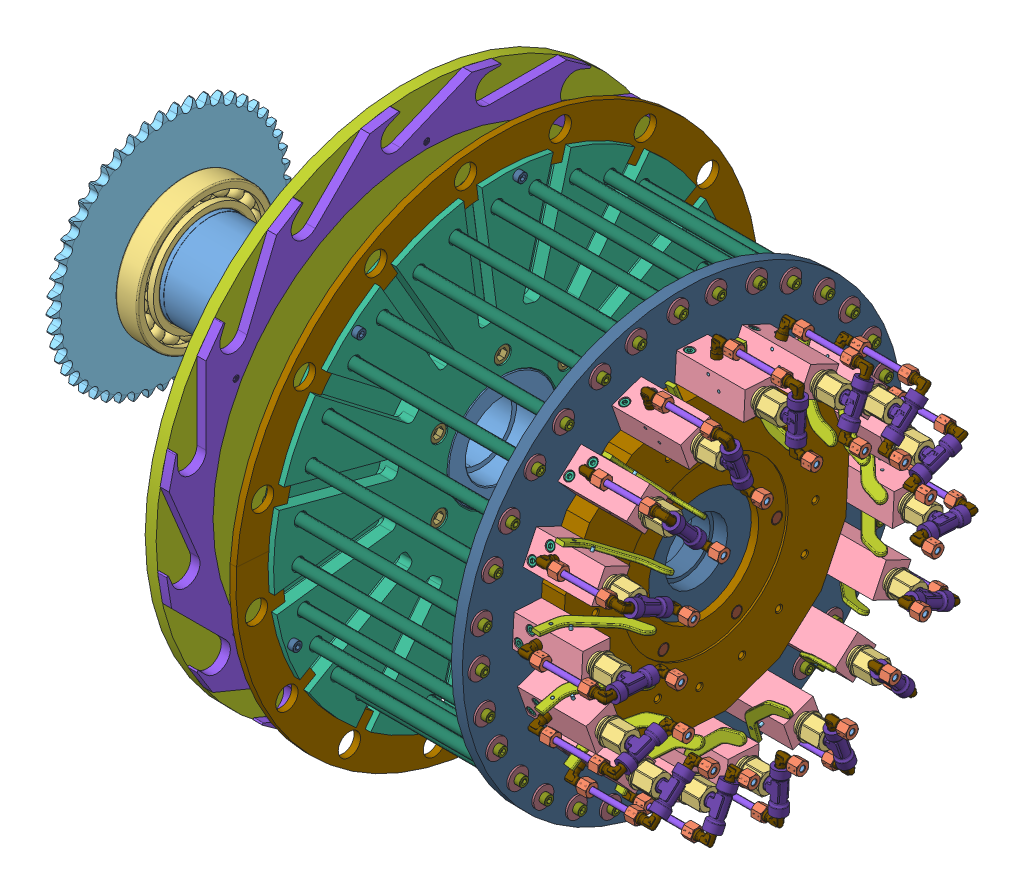
SolidWorks assembly assieme parte rotante, configuration Default. Lengths in mm.
Overall size (749.63 778.63 778.63).
555 component instances, 28 part files, 76 mates.
Components (placement in the parent):
- albero rotazione piatti-1: albero rotazione piatti [Default] at (60.413 18.3637 415) size (415 200 200)
- seger 100mm-1: seger 100mm [KS 1336 E - 100] at (-146.4567 18.3637 415) x (0 0 -1) z (1 0 0) size (107.55 112.98 3)
- SKF - 6020 - 20,DE,NC,20_68-1: SKF - 6020 - 20,DE,NC,20_68 [SKF - 6020 - 20,DE,NC,20_68] at (-131.4567 18.3637 415) x (1 0 0) z (0 -0.434476 -0.900684) size (24 150 150)
- calettatore d95-1: calettatore d95 [Default] at (-173.8867 18.3637 415) size (39.5 135 135)
- Chain wheel ISO - 50Z 10A-1-1: Chain wheel ISO - 50Z 10A-1 [Chain wheel ISO - 50Z 10A-1 --50SB120H25L95.0N] at (-164.8867 18.3637 415) size (28.93 262.06 262.51)
- Disco supporto montaggio e Colonne-1: Disco supporto montaggio e Colonne [Default] at (204.0433 18.3637 415) x (0 -0.866025 -0.5) z (1 0 0) size (499.6 499.6 29)
- SKF - 6020 - 20,DE,NC,20_68-2: SKF - 6020 - 20,DE,NC,20_68 [SKF - 6020 - 20,DE,NC,20_68] at (62.0433 18.3637 415) x (1 0 0) z (0 -0.432628 -0.901573) size (24 150 150)
- piatto rotante porta tappi-1: piatto rotante porta tappi [Default] at (99.0433 18.3637 415) x (0 0 -1) z (1 0 0) size (570 570 20.57)
- disco trasportatore tappi 31-1: disco trasportatore tappi 31 [Default] at (111.0433 18.3637 415) x (0 0.5 -0.866025) z (1 0 0) size (570 570 10.42)
- Distributore Rotante-1: Distributore Rotante [Default] at (425.0433 18.3637 415) x (0 -0.055301 -0.99847) z (1 0 0) size (310 310 25.54)
- disco trascinato porta distributore vuoto-1: disco trascinato porta distributore vuoto [Default] at (400.0433 18.3637 415) x (0 0.055301 0.99847) z (-1 0 0) size (480 480 50)
- m12 35mm-1: m12 35mm [ISO 4762 M12 x 35 - 35N] at (376.0433 -53.0243 378.8925) x (1 0 0) z (0 -0.5 0.866025) size (47 18 18)
- m12 90mm-3: m12 90mm [ISO 4762 M12 x 90 - 90N] at (203.0433 -21.6363 345.718) x (-1 0 0) z (0 -0.5 0.866025) size (102 18 18)
- rondella m6 22mm-1: rondella m6 22mm [Washer ISO 7094 - 6] at (99.0433 -101.6363 207.1539) x (1 0 0) z (0 -1 0) size (2 22 22)
- M6 20mm-1: M6 20mm [ISO 4762 M6 x 20 - 20N] at (91.0433 -101.6363 207.1539) x (1 0 0) z (0 0.5 0.866025) size (26 10 10)
- m12 35mm-2: m12 35mm [ISO 4762 M12 x 35 - 35N] at (376.0433 13.9397 335.1224) x (1 0 0) z (0 -1 0) size (47 18 18)
- m12 35mm-3: m12 35mm [ISO 4762 M12 x 35 - 35N] at (376.0433 85.3277 371.2299) x (1 0 0) z (0 -0.5 -0.866025) size (47 18 18)
- m12 35mm-4: m12 35mm [ISO 4762 M12 x 35 - 35N] at (376.0433 89.7517 451.1075) x (1 0 0) z (0 0.5 -0.866025) size (47 18 18)
- m12 35mm-5: m12 35mm [ISO 4762 M12 x 35 - 35N] at (376.0433 22.7877 494.8776) x (1 0 0) z (0 1 0) size (47 18 18)
- m12 35mm-6: m12 35mm [ISO 4762 M12 x 35 - 35N] at (376.0433 -48.6003 458.7701) x (1 0 0) z (0 0.5 0.866025) size (47 18 18)
- rondella m6 22mm-2: rondella m6 22mm [Washer ISO 7094 - 6] at (99.0433 138.3637 207.1539) x (1 0 0) z (0 -0.5 -0.866025) size (2 22 22)
- rondella m6 22mm-3: rondella m6 22mm [Washer ISO 7094 - 6] at (99.0433 258.3637 415) x (1 0 0) z (0 0.5 -0.866025) size (2 22 22)
- rondella m6 22mm-4: rondella m6 22mm [Washer ISO 7094 - 6] at (99.0433 138.3637 622.8461) x (1 0 0) z (0 1 0) size (2 22 22)
- rondella m6 22mm-5: rondella m6 22mm [Washer ISO 7094 - 6] at (99.0433 -101.6363 622.8461) x (1 0 0) z (0 0.5 0.866025) size (2 22 22)
- rondella m6 22mm-6: rondella m6 22mm [Washer ISO 7094 - 6] at (99.0433 -221.6363 415) x (1 0 0) z (0 -0.5 0.866025) size (2 22 22)
- M6 20mm-2: M6 20mm [ISO 4762 M6 x 20 - 20N] at (91.0433 138.3637 207.1539) x (1 0 0) z (0 -0.5 0.866025) size (26 10 10)
- M6 20mm-3: M6 20mm [ISO 4762 M6 x 20 - 20N] at (91.0433 258.3637 415) x (1 0 0) z (0 -1 0) size (26 10 10)
- M6 20mm-4: M6 20mm [ISO 4762 M6 x 20 - 20N] at (91.0433 138.3637 622.8461) x (1 0 0) z (0 -0.5 -0.866025) size (26 10 10)
- M6 20mm-5: M6 20mm [ISO 4762 M6 x 20 - 20N] at (91.0433 -101.6363 622.8461) x (1 0 0) z (0 0.5 -0.866025) size (26 10 10)
- M6 20mm-6: M6 20mm [ISO 4762 M6 x 20 - 20N] at (91.0433 -221.6363 415) x (1 0 0) z (0 1 0) size (26 10 10)
- m12 90mm-4: m12 90mm [ISO 4762 M12 x 90 - 90N] at (203.0433 58.3637 345.718) x (-1 0 0) z (0 -1 0) size (102 18 18)
- m12 90mm-5: m12 90mm [ISO 4762 M12 x 90 - 90N] at (203.0433 98.3637 415) x (-1 0 0) z (0 -0.5 -0.866025) size (102 18 18)
- m12 90mm-6: m12 90mm [ISO 4762 M12 x 90 - 90N] at (203.0433 58.3637 484.282) x (-1 0 0) z (0 0.5 -0.866025) size (102 18 18)
- m12 90mm-7: m12 90mm [ISO 4762 M12 x 90 - 90N] at (203.0433 -21.6363 484.282) x (-1 0 0) z (0 1 0) size (102 18 18)
- m12 90mm-8: m12 90mm [ISO 4762 M12 x 90 - 90N] at (203.0433 -61.6363 415) x (-1 0 0) z (0 0.5 0.866025) size (102 18 18)
- asta scorrimento carello-1: asta scorrimento carello [Default] at (287.5433 70.1437 197.9013) x (0 0 -1) z (1 0 0) size (12 12 225)
- rondella m6 22mm-7: rondella m6 22mm [Washer ISO 7094 - 6] at (175.0433 70.1437 197.9013) x (1 0 0) z (0 -1 0) size (2 22 22)
- M6 16mm-1: M6 16mm [ISO 4762 M6 x 16 - 16N] at (167.0433 70.1437 197.9013) size (22 10 10)
- M6 16mm-2: M6 16mm [ISO 4762 M6 x 16 - 16N] at (408.0433 70.1437 197.9013) x (-1 0 0) z (0 0 -1) size (22 10 10)
- rondella m6 22mm-8: rondella m6 22mm [Washer ISO 7094 - 6] at (400.0433 70.1437 197.9013) x (-1 0 0) z (0 1 0) size (2 22 22)
- rondella m6 22mm-9: rondella m6 22mm [Washer ISO 7094 - 6] at (175.0433 24.5373 191.8971) x (1 0 0) z (0 -0.965926 -0.258819) size (2 22 22)
- M6 16mm-3: M6 16mm [ISO 4762 M6 x 16 - 16N] at (167.0433 24.5373 191.8971) x (1 0 0) z (0 0.258819 -0.965926) size (22 10 10)
- asta scorrimento carello-2: asta scorrimento carello [Default] at (287.5433 24.5373 191.8971) x (0 0.258819 -0.965926) z (-1 0 0) size (12 12 225)
- rondella m6 22mm-10: rondella m6 22mm [Washer ISO 7094 - 6] at (400.0433 24.5373 191.8971) x (-1 0 0) z (0 0.965926 0.258819) size (2 22 22)
- M6 16mm-4: M6 16mm [ISO 4762 M6 x 16 - 16N] at (408.0433 24.5373 191.8971) x (-1 0 0) z (0 -0.258819 0.965926) size (22 10 10)
- AssiemeValvola-1: AssiemeValvola [Default] at (515.3257 74.6348 254.5832) x (0 -0.331007 0.943628) z (0 0.943628 0.331007) size (90.26 138.63 38)
  - RaccordoT-1: RaccordoT [Default] at origin size (43 29.75 16.5)
  - Raccordo a L-1: Raccordo a L [Default] at (-30 0 0) x (0 -1 0) z (0 0 -1) size (28.34 25.51 14.01)
    - 1809_06_10_01-1: 1809_06_10_01 [Default] at origin size (22.49 23 10)
    - 1809_06_10_02-1: 1809_06_10_02 [Default] at origin size (6.5 8.5 8.5)
    - 1809_06_10_03-1: 1809_06_10_03 [Default] at origin size (11.02 15.01 14.01)
  - Raccordo a L-2: Raccordo a L [Default] at (30 0 0) x (0 1 0) z (0 0 -1) size (28.34 25.51 14.01)
    - 1809_06_10_01-1: 1809_06_10_01 [Default] at origin size (22.49 23 10)
    - 1809_06_10_02-1: 1809_06_10_02 [Default] at origin size (6.5 8.5 8.5)
    - 1809_06_10_03-1: 1809_06_10_03 [Default] at origin size (11.02 15.01 14.01)
  - TappoChiusura-1: TappoChiusura [Default] at (0 -32 0) x (0 -1 0) z (0 0 1) size (38.28 26.74 26.74)
  - CorpoValvola-1: CorpoValvola [Default] at (-15 -115.2824 0) size (30 75 34)
  - Raccordo a L-3: Raccordo a L [Default] at (-30 -88.2824 0) x (0 1 0) z (0 0 1) size (28.34 25.51 14.01)
    - 1809_06_10_01-1: 1809_06_10_01 [Default] at origin size (22.49 23 10)
    - 1809_06_10_02-1: 1809_06_10_02 [Default] at origin size (6.5 8.5 8.5)
    - 1809_06_10_03-1: 1809_06_10_03 [Default] at origin size (11.02 15.01 14.01)
  - Spina_3x38-1: Spina_3x38 [Default] at (0 -68.2824 -21) x (-1 0 0) z (0 0 1) size (3 3 38)
  - Spina_3x38-2: Spina_3x38 [Default] at (-10 -80.2824 -21) x (0.996193 0.087174 0) z (0 0 1) size (3 3 38)
  - M5 40mm-3: M5 40mm [ISO 4762 M5 x 40 - 40N] at (-14.6 -108.7824 9) size (45 8.5 8.5)
  - M5 40mm-2: M5 40mm [ISO 4762 M5 x 40 - 40N] at (-14.6 -96.7824 -9) size (45 8.5 8.5)
  - LevaValvola-1: LevaValvola [Default] at (-24.507 -86.571 -17) x (0.996193 0.087174 0) z (0 0 1) size (77.55 60.2 4)
  - Tubo-1: Tubo [Default] at (-30 -15.9665 0) x (1 0 0) z (0 -1 0) size (6 6 56.4)
- M6 16mm-5: M6 16mm [ISO 4762 M6 x 16 - 16N] at (167.0433 -16.8778 194.6116) x (1 0 0) z (0 0.382683 0.92388) size (22 10 10)
- M6 16mm-6: M6 16mm [ISO 4762 M6 x 16 - 16N] at (167.0433 -98.5342 224.874) x (1 0 0) z (0 0.707107 0.707107) size (22 10 10)
- M6 16mm-7: M6 16mm [ISO 4762 M6 x 16 - 16N] at (167.0433 -162.3939 284.0814) x (1 0 0) z (0 0.92388 0.382683) size (22 10 10)
- M6 16mm-8: M6 16mm [ISO 4762 M6 x 16 - 16N] at (167.0433 -198.735 363.22) x (1 0 0) z (0 1 0) size (22 10 10)
- M6 16mm-9: M6 16mm [ISO 4762 M6 x 16 - 16N] at (167.0433 -202.0247 450.2415) x (1 0 0) z (0 0.92388 -0.382683) size (22 10 10)
- M6 16mm-10: M6 16mm [ISO 4762 M6 x 16 - 16N] at (167.0433 -171.7623 531.8979) x (1 0 0) z (0 0.707107 -0.707107) size (22 10 10)
- M6 16mm-11: M6 16mm [ISO 4762 M6 x 16 - 16N] at (167.0433 -112.5549 595.7576) x (1 0 0) z (0 0.382683 -0.92388) size (22 10 10)
- M6 16mm-12: M6 16mm [ISO 4762 M6 x 16 - 16N] at (167.0433 -33.4163 632.0987) x (1 0 0) z (0 0 -1) size (22 10 10)
- M6 16mm-13: M6 16mm [ISO 4762 M6 x 16 - 16N] at (167.0433 53.6052 635.3884) x (1 0 0) z (0 -0.382683 -0.92388) size (22 10 10)
- M6 16mm-14: M6 16mm [ISO 4762 M6 x 16 - 16N] at (167.0433 135.2616 605.126) x (1 0 0) z (0 -0.707107 -0.707107) size (22 10 10)
- M6 16mm-15: M6 16mm [ISO 4762 M6 x 16 - 16N] at (167.0433 199.1213 545.9186) x (1 0 0) z (0 -0.92388 -0.382683) size (22 10 10)
- M6 16mm-16: M6 16mm [ISO 4762 M6 x 16 - 16N] at (167.0433 235.4624 466.78) x (1 0 0) z (0 -1 0) size (22 10 10)
- M6 16mm-17: M6 16mm [ISO 4762 M6 x 16 - 16N] at (167.0433 238.7521 379.7585) x (1 0 0) z (0 -0.92388 0.382683) size (22 10 10)
- M6 16mm-18: M6 16mm [ISO 4762 M6 x 16 - 16N] at (167.0433 208.4897 298.1021) x (1 0 0) z (0 -0.707107 0.707107) size (22 10 10)
- M6 16mm-19: M6 16mm [ISO 4762 M6 x 16 - 16N] at (167.0433 149.2823 234.2424) x (1 0 0) z (0 -0.382683 0.92388) size (22 10 10)
- rondella m6 22mm-11: rondella m6 22mm [Washer ISO 7094 - 6] at (175.0433 -16.8778 194.6116) x (1 0 0) z (0 -0.92388 0.382683) size (2 22 22)
- rondella m6 22mm-12: rondella m6 22mm [Washer ISO 7094 - 6] at (175.0433 -98.5342 224.874) x (1 0 0) z (0 -0.707107 0.707107) size (2 22 22)
- rondella m6 22mm-13: rondella m6 22mm [Washer ISO 7094 - 6] at (175.0433 -162.3939 284.0814) x (1 0 0) z (0 -0.382683 0.92388) size (2 22 22)
- rondella m6 22mm-14: rondella m6 22mm [Washer ISO 7094 - 6] at (175.0433 -198.735 363.22) size (2 22 22)
- rondella m6 22mm-15: rondella m6 22mm [Washer ISO 7094 - 6] at (175.0433 -202.0247 450.2415) x (1 0 0) z (0 0.382683 0.92388) size (2 22 22)
- rondella m6 22mm-16: rondella m6 22mm [Washer ISO 7094 - 6] at (175.0433 -171.7623 531.8979) x (1 0 0) z (0 0.707107 0.707107) size (2 22 22)
- rondella m6 22mm-17: rondella m6 22mm [Washer ISO 7094 - 6] at (175.0433 -112.5549 595.7576) x (1 0 0) z (0 0.92388 0.382683) size (2 22 22)
- rondella m6 22mm-18: rondella m6 22mm [Washer ISO 7094 - 6] at (175.0433 -33.4163 632.0987) x (1 0 0) z (0 1 0) size (2 22 22)
- rondella m6 22mm-19: rondella m6 22mm [Washer ISO 7094 - 6] at (175.0433 53.6052 635.3884) x (1 0 0) z (0 0.92388 -0.382683) size (2 22 22)
- rondella m6 22mm-20: rondella m6 22mm [Washer ISO 7094 - 6] at (175.0433 135.2616 605.126) x (1 0 0) z (0 0.707107 -0.707107) size (2 22 22)
- rondella m6 22mm-21: rondella m6 22mm [Washer ISO 7094 - 6] at (175.0433 199.1213 545.9186) x (1 0 0) z (0 0.382683 -0.92388) size (2 22 22)
- rondella m6 22mm-22: rondella m6 22mm [Washer ISO 7094 - 6] at (175.0433 235.4624 466.78) x (1 0 0) z (0 0 -1) size (2 22 22)
- rondella m6 22mm-23: rondella m6 22mm [Washer ISO 7094 - 6] at (175.0433 238.7521 379.7585) x (1 0 0) z (0 -0.382683 -0.92388) size (2 22 22)
- rondella m6 22mm-24: rondella m6 22mm [Washer ISO 7094 - 6] at (175.0433 208.4897 298.1021) x (1 0 0) z (0 -0.707107 -0.707107) size (2 22 22)
- rondella m6 22mm-25: rondella m6 22mm [Washer ISO 7094 - 6] at (175.0433 149.2823 234.2424) x (1 0 0) z (0 -0.92388 -0.382683) size (2 22 22)
- asta scorrimento carello-3: asta scorrimento carello [Default] at (287.5433 -16.8778 194.6116) x (0 -0.382683 -0.92388) z (1 0 0) size (12 12 225)
- asta scorrimento carello-4: asta scorrimento carello [Default] at (287.5433 -98.5342 224.874) x (0 -0.707107 -0.707107) z (1 0 0) size (12 12 225)
- asta scorrimento carello-5: asta scorrimento carello [Default] at (287.5433 -162.3939 284.0814) x (0 -0.92388 -0.382683) z (1 0 0) size (12 12 225)
- asta scorrimento carello-6: asta scorrimento carello [Default] at (287.5433 -198.735 363.22) x (0 -1 0) z (1 0 0) size (12 12 225)
- asta scorrimento carello-7: asta scorrimento carello [Default] at (287.5433 -202.0247 450.2415) x (0 -0.92388 0.382683) z (1 0 0) size (12 12 225)
- asta scorrimento carello-8: asta scorrimento carello [Default] at (287.5433 -171.7623 531.8979) x (0 -0.707107 0.707107) z (1 0 0) size (12 12 225)
- asta scorrimento carello-9: asta scorrimento carello [Default] at (287.5433 -112.5549 595.7576) x (0 -0.382683 0.92388) z (1 0 0) size (12 12 225)
- asta scorrimento carello-10: asta scorrimento carello [Default] at (287.5433 -33.4163 632.0987) x (0 0 1) z (1 0 0) size (12 12 225)
- asta scorrimento carello-11: asta scorrimento carello [Default] at (287.5433 53.6052 635.3884) x (0 0.382683 0.92388) z (1 0 0) size (12 12 225)
- asta scorrimento carello-12: asta scorrimento carello [Default] at (287.5433 135.2616 605.126) x (0 0.707107 0.707107) z (1 0 0) size (12 12 225)
- asta scorrimento carello-13: asta scorrimento carello [Default] at (287.5433 199.1213 545.9186) x (0 0.92388 0.382683) z (1 0 0) size (12 12 225)
- asta scorrimento carello-14: asta scorrimento carello [Default] at (287.5433 235.4624 466.78) x (0 1 0) z (1 0 0) size (12 12 225)
- asta scorrimento carello-15: asta scorrimento carello [Default] at (287.5433 238.7521 379.7585) x (0 0.92388 -0.382683) z (1 0 0) size (12 12 225)
- asta scorrimento carello-16: asta scorrimento carello [Default] at (287.5433 208.4897 298.1021) x (0 0.707107 -0.707107) z (1 0 0) size (12 12 225)
- asta scorrimento carello-17: asta scorrimento carello [Default] at (287.5433 149.2823 234.2424) x (0 0.382683 -0.92388) z (1 0 0) size (12 12 225)
- M6 16mm-20: M6 16mm [ISO 4762 M6 x 16 - 16N] at (408.0433 -16.8778 194.6116) x (-1 0 0) z (0 -0.382683 -0.92388) size (22 10 10)
- M6 16mm-21: M6 16mm [ISO 4762 M6 x 16 - 16N] at (408.0433 -98.5342 224.874) x (-1 0 0) z (0 -0.707107 -0.707107) size (22 10 10)
- M6 16mm-22: M6 16mm [ISO 4762 M6 x 16 - 16N] at (408.0433 -162.3939 284.0814) x (-1 0 0) z (0 -0.92388 -0.382683) size (22 10 10)
- M6 16mm-23: M6 16mm [ISO 4762 M6 x 16 - 16N] at (408.0433 -198.735 363.22) x (-1 0 0) z (0 -1 0) size (22 10 10)
- M6 16mm-24: M6 16mm [ISO 4762 M6 x 16 - 16N] at (408.0433 -202.0247 450.2415) x (-1 0 0) z (0 -0.92388 0.382683) size (22 10 10)
- M6 16mm-25: M6 16mm [ISO 4762 M6 x 16 - 16N] at (408.0433 -171.7623 531.8979) x (-1 0 0) z (0 -0.707107 0.707107) size (22 10 10)
- M6 16mm-26: M6 16mm [ISO 4762 M6 x 16 - 16N] at (408.0433 -112.5549 595.7576) x (-1 0 0) z (0 -0.382683 0.92388) size (22 10 10)
- M6 16mm-27: M6 16mm [ISO 4762 M6 x 16 - 16N] at (408.0433 -33.4163 632.0987) x (-1 0 0) z (0 0 1) size (22 10 10)
- M6 16mm-28: M6 16mm [ISO 4762 M6 x 16 - 16N] at (408.0433 53.6052 635.3884) x (-1 0 0) z (0 0.382683 0.92388) size (22 10 10)
- M6 16mm-29: M6 16mm [ISO 4762 M6 x 16 - 16N] at (408.0433 135.2616 605.126) x (-1 0 0) z (0 0.707107 0.707107) size (22 10 10)
- M6 16mm-30: M6 16mm [ISO 4762 M6 x 16 - 16N] at (408.0433 199.1213 545.9186) x (-1 0 0) z (0 0.92388 0.382683) size (22 10 10)
- M6 16mm-31: M6 16mm [ISO 4762 M6 x 16 - 16N] at (408.0433 235.4624 466.78) x (-1 0 0) z (0 1 0) size (22 10 10)
- M6 16mm-32: M6 16mm [ISO 4762 M6 x 16 - 16N] at (408.0433 238.7521 379.7585) x (-1 0 0) z (0 0.92388 -0.382683) size (22 10 10)
- M6 16mm-33: M6 16mm [ISO 4762 M6 x 16 - 16N] at (408.0433 208.4897 298.1021) x (-1 0 0) z (0 0.707107 -0.707107) size (22 10 10)
- M6 16mm-34: M6 16mm [ISO 4762 M6 x 16 - 16N] at (408.0433 149.2823 234.2424) x (-1 0 0) z (0 0.382683 -0.92388) size (22 10 10)
- rondella m6 22mm-26: rondella m6 22mm [Washer ISO 7094 - 6] at (400.0433 -16.8778 194.6116) x (-1 0 0) z (0 0.92388 -0.382683) size (2 22 22)
- rondella m6 22mm-27: rondella m6 22mm [Washer ISO 7094 - 6] at (400.0433 -98.5342 224.874) x (-1 0 0) z (0 0.707107 -0.707107) size (2 22 22)
- rondella m6 22mm-28: rondella m6 22mm [Washer ISO 7094 - 6] at (400.0433 -162.3939 284.0814) x (-1 0 0) z (0 0.382683 -0.92388) size (2 22 22)
- rondella m6 22mm-29: rondella m6 22mm [Washer ISO 7094 - 6] at (400.0433 -198.735 363.22) x (-1 0 0) z (0 0 -1) size (2 22 22)
- rondella m6 22mm-30: rondella m6 22mm [Washer ISO 7094 - 6] at (400.0433 -202.0247 450.2415) x (-1 0 0) z (0 -0.382683 -0.92388) size (2 22 22)
- rondella m6 22mm-31: rondella m6 22mm [Washer ISO 7094 - 6] at (400.0433 -171.7623 531.8979) x (-1 0 0) z (0 -0.707107 -0.707107) size (2 22 22)
- rondella m6 22mm-32: rondella m6 22mm [Washer ISO 7094 - 6] at (400.0433 -112.5549 595.7576) x (-1 0 0) z (0 -0.92388 -0.382683) size (2 22 22)
- rondella m6 22mm-33: rondella m6 22mm [Washer ISO 7094 - 6] at (400.0433 -33.4163 632.0987) x (-1 0 0) z (0 -1 0) size (2 22 22)
- rondella m6 22mm-34: rondella m6 22mm [Washer ISO 7094 - 6] at (400.0433 53.6052 635.3884) x (-1 0 0) z (0 -0.92388 0.382683) size (2 22 22)
- rondella m6 22mm-35: rondella m6 22mm [Washer ISO 7094 - 6] at (400.0433 135.2616 605.126) x (-1 0 0) z (0 -0.707107 0.707107) size (2 22 22)
- rondella m6 22mm-36: rondella m6 22mm [Washer ISO 7094 - 6] at (400.0433 199.1213 545.9186) x (-1 0 0) z (0 -0.382683 0.92388) size (2 22 22)
- rondella m6 22mm-37: rondella m6 22mm [Washer ISO 7094 - 6] at (400.0433 235.4624 466.78) x (-1 0 0) z (0 0 1) size (2 22 22)
- rondella m6 22mm-38: rondella m6 22mm [Washer ISO 7094 - 6] at (400.0433 238.7521 379.7585) x (-1 0 0) z (0 0.382683 0.92388) size (2 22 22)
- rondella m6 22mm-39: rondella m6 22mm [Washer ISO 7094 - 6] at (400.0433 208.4897 298.1021) x (-1 0 0) z (0 0.707107 0.707107) size (2 22 22)
- rondella m6 22mm-40: rondella m6 22mm [Washer ISO 7094 - 6] at (400.0433 149.2823 234.2424) x (-1 0 0) z (0 0.92388 0.382683) size (2 22 22)
- rondella m6 22mm-41: rondella m6 22mm [Washer ISO 7094 - 6] at (175.0433 -61.3104 206.5173) x (1 0 0) z (0 -0.991445 0.130526) size (2 22 22)
- rondella m6 22mm-42: rondella m6 22mm [Washer ISO 7094 - 6] at (175.0433 -135.0285 252.8771) x (1 0 0) z (0 -0.866025 0.5) size (2 22 22)
- rondella m6 22mm-43: rondella m6 22mm [Washer ISO 7094 - 6] at (175.0433 -185.3939 323.9186) x (1 0 0) z (0 -0.608761 0.793353) size (2 22 22)
- rondella m6 22mm-44: rondella m6 22mm [Washer ISO 7094 - 6] at (175.0433 -204.7392 408.8264) x (1 0 0) z (0 -0.258819 0.965926) size (2 22 22)
- rondella m6 22mm-45: rondella m6 22mm [Washer ISO 7094 - 6] at (175.0433 -190.119 494.6741) x (1 0 0) z (0 0.130526 0.991445) size (2 22 22)
- rondella m6 22mm-46: rondella m6 22mm [Washer ISO 7094 - 6] at (175.0433 -143.7592 568.3922) x (1 0 0) z (0 0.5 0.866025) size (2 22 22)
- rondella m6 22mm-47: rondella m6 22mm [Washer ISO 7094 - 6] at (175.0433 -72.7177 618.7576) x (1 0 0) z (0 0.793353 0.608761) size (2 22 22)
- rondella m6 22mm-48: rondella m6 22mm [Washer ISO 7094 - 6] at (175.0433 12.1901 638.1029) x (1 0 0) z (0 0.965926 0.258819) size (2 22 22)
- rondella m6 22mm-49: rondella m6 22mm [Washer ISO 7094 - 6] at (175.0433 98.0378 623.4827) x (1 0 0) z (0 0.991445 -0.130526) size (2 22 22)
- rondella m6 22mm-50: rondella m6 22mm [Washer ISO 7094 - 6] at (175.0433 171.7559 577.1229) x (1 0 0) z (0 0.866025 -0.5) size (2 22 22)
- rondella m6 22mm-51: rondella m6 22mm [Washer ISO 7094 - 6] at (175.0433 222.1213 506.0814) x (1 0 0) z (0 0.608761 -0.793353) size (2 22 22)
- rondella m6 22mm-52: rondella m6 22mm [Washer ISO 7094 - 6] at (175.0433 241.4666 421.1736) x (1 0 0) z (0 0.258819 -0.965926) size (2 22 22)
- rondella m6 22mm-53: rondella m6 22mm [Washer ISO 7094 - 6] at (175.0433 226.8464 335.3259) x (1 0 0) z (0 -0.130526 -0.991445) size (2 22 22)
- rondella m6 22mm-54: rondella m6 22mm [Washer ISO 7094 - 6] at (175.0433 180.4866 261.6078) x (1 0 0) z (0 -0.5 -0.866025) size (2 22 22)
- rondella m6 22mm-55: rondella m6 22mm [Washer ISO 7094 - 6] at (175.0433 109.4451 211.2424) x (1 0 0) z (0 -0.793353 -0.608761) size (2 22 22)
- M6 16mm-35: M6 16mm [ISO 4762 M6 x 16 - 16N] at (167.0433 -61.3104 206.5173) x (1 0 0) z (0 -0.130526 -0.991445) size (22 10 10)
- M6 16mm-36: M6 16mm [ISO 4762 M6 x 16 - 16N] at (167.0433 -135.0285 252.8771) x (1 0 0) z (0 -0.5 -0.866025) size (22 10 10)
- M6 16mm-37: M6 16mm [ISO 4762 M6 x 16 - 16N] at (167.0433 -185.3939 323.9186) x (1 0 0) z (0 -0.793353 -0.608761) size (22 10 10)
- M6 16mm-38: M6 16mm [ISO 4762 M6 x 16 - 16N] at (167.0433 -204.7392 408.8264) x (1 0 0) z (0 -0.965926 -0.258819) size (22 10 10)
- M6 16mm-39: M6 16mm [ISO 4762 M6 x 16 - 16N] at (167.0433 -190.119 494.6741) x (1 0 0) z (0 -0.991445 0.130526) size (22 10 10)
- M6 16mm-40: M6 16mm [ISO 4762 M6 x 16 - 16N] at (167.0433 -143.7592 568.3922) x (1 0 0) z (0 -0.866025 0.5) size (22 10 10)
- M6 16mm-41: M6 16mm [ISO 4762 M6 x 16 - 16N] at (167.0433 -72.7177 618.7576) x (1 0 0) z (0 -0.608761 0.793353) size (22 10 10)
- M6 16mm-42: M6 16mm [ISO 4762 M6 x 16 - 16N] at (167.0433 12.1901 638.1029) x (1 0 0) z (0 -0.258819 0.965926) size (22 10 10)
- M6 16mm-43: M6 16mm [ISO 4762 M6 x 16 - 16N] at (167.0433 98.0378 623.4827) x (1 0 0) z (0 0.130526 0.991445) size (22 10 10)
- M6 16mm-44: M6 16mm [ISO 4762 M6 x 16 - 16N] at (167.0433 171.7559 577.1229) x (1 0 0) z (0 0.5 0.866025) size (22 10 10)
- M6 16mm-45: M6 16mm [ISO 4762 M6 x 16 - 16N] at (167.0433 222.1213 506.0814) x (1 0 0) z (0 0.793353 0.608761) size (22 10 10)
- M6 16mm-46: M6 16mm [ISO 4762 M6 x 16 - 16N] at (167.0433 241.4666 421.1736) x (1 0 0) z (0 0.965926 0.258819) size (22 10 10)
- M6 16mm-47: M6 16mm [ISO 4762 M6 x 16 - 16N] at (167.0433 226.8464 335.3259) x (1 0 0) z (0 0.991445 -0.130526) size (22 10 10)
- M6 16mm-48: M6 16mm [ISO 4762 M6 x 16 - 16N] at (167.0433 180.4866 261.6078) x (1 0 0) z (0 0.866025 -0.5) size (22 10 10)
- M6 16mm-49: M6 16mm [ISO 4762 M6 x 16 - 16N] at (167.0433 109.4451 211.2424) x (1 0 0) z (0 0.608761 -0.793353) size (22 10 10)
- asta scorrimento carello-18: asta scorrimento carello [Default] at (287.5433 -61.3104 206.5173) x (0 -0.130526 -0.991445) z (-1 0 0) size (12 12 225)
- asta scorrimento carello-19: asta scorrimento carello [Default] at (287.5433 -135.0285 252.8771) x (0 -0.5 -0.866025) z (-1 0 0) size (12 12 225)
- asta scorrimento carello-20: asta scorrimento carello [Default] at (287.5433 -185.3939 323.9186) x (0 -0.793353 -0.608761) z (-1 0 0) size (12 12 225)
- asta scorrimento carello-21: asta scorrimento carello [Default] at (287.5433 -204.7392 408.8264) x (0 -0.965926 -0.258819) z (-1 0 0) size (12 12 225)
- asta scorrimento carello-22: asta scorrimento carello [Default] at (287.5433 -190.119 494.6741) x (0 -0.991445 0.130526) z (-1 0 0) size (12 12 225)
- asta scorrimento carello-23: asta scorrimento carello [Default] at (287.5433 -143.7592 568.3922) x (0 -0.866025 0.5) z (-1 0 0) size (12 12 225)
- asta scorrimento carello-24: asta scorrimento carello [Default] at (287.5433 -72.7177 618.7576) x (0 -0.608761 0.793353) z (-1 0 0) size (12 12 225)
- asta scorrimento carello-25: asta scorrimento carello [Default] at (287.5433 12.1901 638.1029) x (0 -0.258819 0.965926) z (-1 0 0) size (12 12 225)
- asta scorrimento carello-26: asta scorrimento carello [Default] at (287.5433 98.0378 623.4827) x (0 0.130526 0.991445) z (-1 0 0) size (12 12 225)
- asta scorrimento carello-27: asta scorrimento carello [Default] at (287.5433 171.7559 577.1229) x (0 0.5 0.866025) z (-1 0 0) size (12 12 225)
- asta scorrimento carello-28: asta scorrimento carello [Default] at (287.5433 222.1213 506.0814) x (0 0.793353 0.608761) z (-1 0 0) size (12 12 225)
- asta scorrimento carello-29: asta scorrimento carello [Default] at (287.5433 241.4666 421.1736) x (0 0.965926 0.258819) z (-1 0 0) size (12 12 225)
- asta scorrimento carello-30: asta scorrimento carello [Default] at (287.5433 226.8464 335.3259) x (0 0.991445 -0.130526) z (-1 0 0) size (12 12 225)
- asta scorrimento carello-31: asta scorrimento carello [Default] at (287.5433 180.4866 261.6078) x (0 0.866025 -0.5) z (-1 0 0) size (12 12 225)
- asta scorrimento carello-32: asta scorrimento carello [Default] at (287.5433 109.4451 211.2424) x (0 0.608761 -0.793353) z (-1 0 0) size (12 12 225)
- rondella m6 22mm-56: rondella m6 22mm [Washer ISO 7094 - 6] at (400.0433 -61.3104 206.5173) x (-1 0 0) z (0 0.991445 -0.130526) size (2 22 22)
- rondella m6 22mm-57: rondella m6 22mm [Washer ISO 7094 - 6] at (400.0433 -135.0285 252.8771) x (-1 0 0) z (0 0.866025 -0.5) size (2 22 22)
- rondella m6 22mm-58: rondella m6 22mm [Washer ISO 7094 - 6] at (400.0433 -185.3939 323.9186) x (-1 0 0) z (0 0.608761 -0.793353) size (2 22 22)
- rondella m6 22mm-59: rondella m6 22mm [Washer ISO 7094 - 6] at (400.0433 -204.7392 408.8264) x (-1 0 0) z (0 0.258819 -0.965926) size (2 22 22)
- rondella m6 22mm-60: rondella m6 22mm [Washer ISO 7094 - 6] at (400.0433 -190.119 494.6741) x (-1 0 0) z (0 -0.130526 -0.991445) size (2 22 22)
- rondella m6 22mm-61: rondella m6 22mm [Washer ISO 7094 - 6] at (400.0433 -143.7592 568.3922) x (-1 0 0) z (0 -0.5 -0.866025) size (2 22 22)
- rondella m6 22mm-62: rondella m6 22mm [Washer ISO 7094 - 6] at (400.0433 -72.7177 618.7576) x (-1 0 0) z (0 -0.793353 -0.608761) size (2 22 22)
- rondella m6 22mm-63: rondella m6 22mm [Washer ISO 7094 - 6] at (400.0433 12.1901 638.1029) x (-1 0 0) z (0 -0.965926 -0.258819) size (2 22 22)
- rondella m6 22mm-64: rondella m6 22mm [Washer ISO 7094 - 6] at (400.0433 98.0378 623.4827) x (-1 0 0) z (0 -0.991445 0.130526) size (2 22 22)
- rondella m6 22mm-65: rondella m6 22mm [Washer ISO 7094 - 6] at (400.0433 171.7559 577.1229) x (-1 0 0) z (0 -0.866025 0.5) size (2 22 22)
- rondella m6 22mm-66: rondella m6 22mm [Washer ISO 7094 - 6] at (400.0433 222.1213 506.0814) x (-1 0 0) z (0 -0.608761 0.793353) size (2 22 22)
- rondella m6 22mm-67: rondella m6 22mm [Washer ISO 7094 - 6] at (400.0433 241.4666 421.1736) x (-1 0 0) z (0 -0.258819 0.965926) size (2 22 22)
- rondella m6 22mm-68: rondella m6 22mm [Washer ISO 7094 - 6] at (400.0433 226.8464 335.3259) x (-1 0 0) z (0 0.130526 0.991445) size (2 22 22)
- rondella m6 22mm-69: rondella m6 22mm [Washer ISO 7094 - 6] at (400.0433 180.4866 261.6078) x (-1 0 0) z (0 0.5 0.866025) size (2 22 22)
- rondella m6 22mm-70: rondella m6 22mm [Washer ISO 7094 - 6] at (400.0433 109.4451 211.2424) x (-1 0 0) z (0 0.793353 0.608761) size (2 22 22)
- M6 16mm-50: M6 16mm [ISO 4762 M6 x 16 - 16N] at (408.0433 -61.3104 206.5173) x (-1 0 0) z (0 0.130526 0.991445) size (22 10 10)
- M6 16mm-51: M6 16mm [ISO 4762 M6 x 16 - 16N] at (408.0433 -135.0285 252.8771) x (-1 0 0) z (0 0.5 0.866025) size (22 10 10)
- M6 16mm-52: M6 16mm [ISO 4762 M6 x 16 - 16N] at (408.0433 -185.3939 323.9186) x (-1 0 0) z (0 0.793353 0.608761) size (22 10 10)
- M6 16mm-53: M6 16mm [ISO 4762 M6 x 16 - 16N] at (408.0433 -204.7392 408.8264) x (-1 0 0) z (0 0.965926 0.258819) size (22 10 10)
- M6 16mm-54: M6 16mm [ISO 4762 M6 x 16 - 16N] at (408.0433 -190.119 494.6741) x (-1 0 0) z (0 0.991445 -0.130526) size (22 10 10)
- M6 16mm-55: M6 16mm [ISO 4762 M6 x 16 - 16N] at (408.0433 -143.7592 568.3922) x (-1 0 0) z (0 0.866025 -0.5) size (22 10 10)
- M6 16mm-56: M6 16mm [ISO 4762 M6 x 16 - 16N] at (408.0433 -72.7177 618.7576) x (-1 0 0) z (0 0.608761 -0.793353) size (22 10 10)
- M6 16mm-57: M6 16mm [ISO 4762 M6 x 16 - 16N] at (408.0433 12.1901 638.1029) x (-1 0 0) z (0 0.258819 -0.965926) size (22 10 10)
- M6 16mm-58: M6 16mm [ISO 4762 M6 x 16 - 16N] at (408.0433 98.0378 623.4827) x (-1 0 0) z (0 -0.130526 -0.991445) size (22 10 10)
- M6 16mm-59: M6 16mm [ISO 4762 M6 x 16 - 16N] at (408.0433 171.7559 577.1229) x (-1 0 0) z (0 -0.5 -0.866025) size (22 10 10)
- M6 16mm-60: M6 16mm [ISO 4762 M6 x 16 - 16N] at (408.0433 222.1213 506.0814) x (-1 0 0) z (0 -0.793353 -0.608761) size (22 10 10)
- M6 16mm-61: M6 16mm [ISO 4762 M6 x 16 - 16N] at (408.0433 241.4666 421.1736) x (-1 0 0) z (0 -0.965926 -0.258819) size (22 10 10)
- M6 16mm-62: M6 16mm [ISO 4762 M6 x 16 - 16N] at (408.0433 226.8464 335.3259) x (-1 0 0) z (0 -0.991445 0.130526) size (22 10 10)
- M6 16mm-63: M6 16mm [ISO 4762 M6 x 16 - 16N] at (408.0433 180.4866 261.6078) x (-1 0 0) z (0 -0.866025 0.5) size (22 10 10)
- M6 16mm-64: M6 16mm [ISO 4762 M6 x 16 - 16N] at (408.0433 109.4451 211.2424) x (-1 0 0) z (0 -0.608761 0.793353) size (22 10 10)
- AssiemeValvola-2: AssiemeValvola [Default] at (515.3257 8.9626 245.2601) x (0 0.055301 0.99847) z (0 0.99847 -0.055301) size (90.26 138.63 38)
  - RaccordoT-1: RaccordoT [Default] at origin size (43 29.75 16.5)
  - Raccordo a L-1: Raccordo a L [Default] at (-30 0 0) x (0 -1 0) z (0 0 -1) size (28.34 25.51 14.01)
    - 1809_06_10_01-1: 1809_06_10_01 [Default] at origin size (22.49 23 10)
    - 1809_06_10_02-1: 1809_06_10_02 [Default] at origin size (6.5 8.5 8.5)
    - 1809_06_10_03-1: 1809_06_10_03 [Default] at origin size (11.02 15.01 14.01)
  - Raccordo a L-2: Raccordo a L [Default] at (30 0 0) x (0 1 0) z (0 0 -1) size (28.34 25.51 14.01)
    - 1809_06_10_01-1: 1809_06_10_01 [Default] at origin size (22.49 23 10)
    - 1809_06_10_02-1: 1809_06_10_02 [Default] at origin size (6.5 8.5 8.5)
    - 1809_06_10_03-1: 1809_06_10_03 [Default] at origin size (11.02 15.01 14.01)
  - TappoChiusura-1: TappoChiusura [Default] at (0 -32 0) x (0 -1 0) z (0 0 1) size (38.28 26.74 26.74)
  - CorpoValvola-1: CorpoValvola [Default] at (-15 -115.2824 0) size (30 75 34)
  - Raccordo a L-3: Raccordo a L [Default] at (-30 -88.2824 0) x (0 1 0) z (0 0 1) size (28.34 25.51 14.01)
    - 1809_06_10_01-1: 1809_06_10_01 [Default] at origin size (22.49 23 10)
    - 1809_06_10_02-1: 1809_06_10_02 [Default] at origin size (6.5 8.5 8.5)
    - 1809_06_10_03-1: 1809_06_10_03 [Default] at origin size (11.02 15.01 14.01)
  - Spina_3x38-1: Spina_3x38 [Default] at (0 -68.2824 -21) x (-1 0 0) z (0 0 1) size (3 3 38)
  - Spina_3x38-2: Spina_3x38 [Default] at (-10 -80.2824 -21) x (0.996193 0.087174 0) z (0 0 1) size (3 3 38)
  - M5 40mm-3: M5 40mm [ISO 4762 M5 x 40 - 40N] at (-14.6 -108.7824 9) size (45 8.5 8.5)
  - M5 40mm-2: M5 40mm [ISO 4762 M5 x 40 - 40N] at (-14.6 -96.7824 -9) size (45 8.5 8.5)
  - LevaValvola-1: LevaValvola [Default] at (-24.507 -86.571 -17) x (0.996193 0.087174 0) z (0 0 1) size (77.55 60.2 4)
  - Tubo-1: Tubo [Default] at (-30 -15.9665 0) x (1 0 0) z (0 -1 0) size (6 6 56.4)
- AssiemeValvola-3: AssiemeValvola [Default] at (515.3257 -55.2784 261.7785) x (0 0.433189 0.901303) z (0 0.901303 -0.433189) size (90.26 138.63 38)
  - RaccordoT-1: RaccordoT [Default] at origin size (43 29.75 16.5)
  - Raccordo a L-1: Raccordo a L [Default] at (-30 0 0) x (0 -1 0) z (0 0 -1) size (28.34 25.51 14.01)
    - 1809_06_10_01-1: 1809_06_10_01 [Default] at origin size (22.49 23 10)
    - 1809_06_10_02-1: 1809_06_10_02 [Default] at origin size (6.5 8.5 8.5)
    - 1809_06_10_03-1: 1809_06_10_03 [Default] at origin size (11.02 15.01 14.01)
  - Raccordo a L-2: Raccordo a L [Default] at (30 0 0) x (0 1 0) z (0 0 -1) size (28.34 25.51 14.01)
    - 1809_06_10_01-1: 1809_06_10_01 [Default] at origin size (22.49 23 10)
    - 1809_06_10_02-1: 1809_06_10_02 [Default] at origin size (6.5 8.5 8.5)
    - 1809_06_10_03-1: 1809_06_10_03 [Default] at origin size (11.02 15.01 14.01)
  - TappoChiusura-1: TappoChiusura [Default] at (0 -32 0) x (0 -1 0) z (0 0 1) size (38.28 26.74 26.74)
  - CorpoValvola-1: CorpoValvola [Default] at (-15 -115.2824 0) size (30 75 34)
  - Raccordo a L-3: Raccordo a L [Default] at (-30 -88.2824 0) x (0 1 0) z (0 0 1) size (28.34 25.51 14.01)
    - 1809_06_10_01-1: 1809_06_10_01 [Default] at origin size (22.49 23 10)
    - 1809_06_10_02-1: 1809_06_10_02 [Default] at origin size (6.5 8.5 8.5)
    - 1809_06_10_03-1: 1809_06_10_03 [Default] at origin size (11.02 15.01 14.01)
  - Spina_3x38-1: Spina_3x38 [Default] at (0 -68.2824 -21) x (-1 0 0) z (0 0 1) size (3 3 38)
  - Spina_3x38-2: Spina_3x38 [Default] at (-10 -80.2824 -21) x (0.996193 0.087174 0) z (0 0 1) size (3 3 38)
  - M5 40mm-3: M5 40mm [ISO 4762 M5 x 40 - 40N] at (-14.6 -108.7824 9) size (45 8.5 8.5)
  - M5 40mm-2: M5 40mm [ISO 4762 M5 x 40 - 40N] at (-14.6 -96.7824 -9) size (45 8.5 8.5)
  - LevaValvola-1: LevaValvola [Default] at (-24.507 -86.571 -17) x (0.996193 0.087174 0) z (0 0 1) size (77.55 60.2 4)
  - Tubo-1: Tubo [Default] at (-30 -15.9665 0) x (1 0 0) z (0 -1 0) size (6 6 56.4)
- AssiemeValvola-4: AssiemeValvola [Default] at (515.3257 -108.3081 301.6234) x (0 0.745128 0.666921) z (0 0.666921 -0.745128) size (90.26 138.63 38)
  - RaccordoT-1: RaccordoT [Default] at origin size (43 29.75 16.5)
  - Raccordo a L-1: Raccordo a L [Default] at (-30 0 0) x (0 -1 0) z (0 0 -1) size (28.34 25.51 14.01)
    - 1809_06_10_01-1: 1809_06_10_01 [Default] at origin size (22.49 23 10)
    - 1809_06_10_02-1: 1809_06_10_02 [Default] at origin size (6.5 8.5 8.5)
    - 1809_06_10_03-1: 1809_06_10_03 [Default] at origin size (11.02 15.01 14.01)
  - Raccordo a L-2: Raccordo a L [Default] at (30 0 0) x (0 1 0) z (0 0 -1) size (28.34 25.51 14.01)
    - 1809_06_10_01-1: 1809_06_10_01 [Default] at origin size (22.49 23 10)
    - 1809_06_10_02-1: 1809_06_10_02 [Default] at origin size (6.5 8.5 8.5)
    - 1809_06_10_03-1: 1809_06_10_03 [Default] at origin size (11.02 15.01 14.01)
  - TappoChiusura-1: TappoChiusura [Default] at (0 -32 0) x (0 -1 0) z (0 0 1) size (38.28 26.74 26.74)
  - CorpoValvola-1: CorpoValvola [Default] at (-15 -115.2824 0) size (30 75 34)
  - Raccordo a L-3: Raccordo a L [Default] at (-30 -88.2824 0) x (0 1 0) z (0 0 1) size (28.34 25.51 14.01)
    - 1809_06_10_01-1: 1809_06_10_01 [Default] at origin size (22.49 23 10)
    - 1809_06_10_02-1: 1809_06_10_02 [Default] at origin size (6.5 8.5 8.5)
    - 1809_06_10_03-1: 1809_06_10_03 [Default] at origin size (11.02 15.01 14.01)
  - Spina_3x38-1: Spina_3x38 [Default] at (0 -68.2824 -21) x (-1 0 0) z (0 0 1) size (3 3 38)
  - Spina_3x38-2: Spina_3x38 [Default] at (-10 -80.2824 -21) x (0.996193 0.087174 0) z (0 0 1) size (3 3 38)
  - M5 40mm-3: M5 40mm [ISO 4762 M5 x 40 - 40N] at (-14.6 -108.7824 9) size (45 8.5 8.5)
  - M5 40mm-2: M5 40mm [ISO 4762 M5 x 40 - 40N] at (-14.6 -96.7824 -9) size (45 8.5 8.5)
  - LevaValvola-1: LevaValvola [Default] at (-24.507 -86.571 -17) x (0.996193 0.087174 0) z (0 0 1) size (77.55 60.2 4)
  - Tubo-1: Tubo [Default] at (-30 -15.9665 0) x (1 0 0) z (0 -1 0) size (6 6 56.4)
- AssiemeValvola-5: AssiemeValvola [Default] at (515.3257 -142.0531 358.7289) x (0 0.943628 0.331007) z (0 0.331007 -0.943628) size (90.26 138.63 38)
  - RaccordoT-1: RaccordoT [Default] at origin size (43 29.75 16.5)
  - Raccordo a L-1: Raccordo a L [Default] at (-30 0 0) x (0 -1 0) z (0 0 -1) size (28.34 25.51 14.01)
    - 1809_06_10_01-1: 1809_06_10_01 [Default] at origin size (22.49 23 10)
    - 1809_06_10_02-1: 1809_06_10_02 [Default] at origin size (6.5 8.5 8.5)
    - 1809_06_10_03-1: 1809_06_10_03 [Default] at origin size (11.02 15.01 14.01)
  - Raccordo a L-2: Raccordo a L [Default] at (30 0 0) x (0 1 0) z (0 0 -1) size (28.34 25.51 14.01)
    - 1809_06_10_01-1: 1809_06_10_01 [Default] at origin size (22.49 23 10)
    - 1809_06_10_02-1: 1809_06_10_02 [Default] at origin size (6.5 8.5 8.5)
    - 1809_06_10_03-1: 1809_06_10_03 [Default] at origin size (11.02 15.01 14.01)
  - TappoChiusura-1: TappoChiusura [Default] at (0 -32 0) x (0 -1 0) z (0 0 1) size (38.28 26.74 26.74)
  - CorpoValvola-1: CorpoValvola [Default] at (-15 -115.2824 0) size (30 75 34)
  - Raccordo a L-3: Raccordo a L [Default] at (-30 -88.2824 0) x (0 1 0) z (0 0 1) size (28.34 25.51 14.01)
    - 1809_06_10_01-1: 1809_06_10_01 [Default] at origin size (22.49 23 10)
    - 1809_06_10_02-1: 1809_06_10_02 [Default] at origin size (6.5 8.5 8.5)
    - 1809_06_10_03-1: 1809_06_10_03 [Default] at origin size (11.02 15.01 14.01)
  - Spina_3x38-1: Spina_3x38 [Default] at (0 -68.2824 -21) x (-1 0 0) z (0 0 1) size (3 3 38)
  - Spina_3x38-2: Spina_3x38 [Default] at (-10 -80.2824 -21) x (0.996193 0.087174 0) z (0 0 1) size (3 3 38)
  - M5 40mm-3: M5 40mm [ISO 4762 M5 x 40 - 40N] at (-14.6 -108.7824 9) size (45 8.5 8.5)
  - M5 40mm-2: M5 40mm [ISO 4762 M5 x 40 - 40N] at (-14.6 -96.7824 -9) size (45 8.5 8.5)
  - LevaValvola-1: LevaValvola [Default] at (-24.507 -86.571 -17) x (0.996193 0.087174 0) z (0 0 1) size (77.55 60.2 4)
  - Tubo-1: Tubo [Default] at (-30 -15.9665 0) x (1 0 0) z (0 -1 0) size (6 6 56.4)
- AssiemeValvola-6: AssiemeValvola [Default] at (515.3257 -151.3762 424.4011) x (0 0.99847 -0.055301) z (0 -0.055301 -0.99847) size (90.26 138.63 38)
  - RaccordoT-1: RaccordoT [Default] at origin size (43 29.75 16.5)
  - Raccordo a L-1: Raccordo a L [Default] at (-30 0 0) x (0 -1 0) z (0 0 -1) size (28.34 25.51 14.01)
    - 1809_06_10_01-1: 1809_06_10_01 [Default] at origin size (22.49 23 10)
    - 1809_06_10_02-1: 1809_06_10_02 [Default] at origin size (6.5 8.5 8.5)
    - 1809_06_10_03-1: 1809_06_10_03 [Default] at origin size (11.02 15.01 14.01)
  - Raccordo a L-2: Raccordo a L [Default] at (30 0 0) x (0 1 0) z (0 0 -1) size (28.34 25.51 14.01)
    - 1809_06_10_01-1: 1809_06_10_01 [Default] at origin size (22.49 23 10)
    - 1809_06_10_02-1: 1809_06_10_02 [Default] at origin size (6.5 8.5 8.5)
    - 1809_06_10_03-1: 1809_06_10_03 [Default] at origin size (11.02 15.01 14.01)
  - TappoChiusura-1: TappoChiusura [Default] at (0 -32 0) x (0 -1 0) z (0 0 1) size (38.28 26.74 26.74)
  - CorpoValvola-1: CorpoValvola [Default] at (-15 -115.2824 0) size (30 75 34)
  - Raccordo a L-3: Raccordo a L [Default] at (-30 -88.2824 0) x (0 1 0) z (0 0 1) size (28.34 25.51 14.01)
    - 1809_06_10_01-1: 1809_06_10_01 [Default] at origin size (22.49 23 10)
    - 1809_06_10_02-1: 1809_06_10_02 [Default] at origin size (6.5 8.5 8.5)
    - 1809_06_10_03-1: 1809_06_10_03 [Default] at origin size (11.02 15.01 14.01)
  - Spina_3x38-1: Spina_3x38 [Default] at (0 -68.2824 -21) x (-1 0 0) z (0 0 1) size (3 3 38)
  - Spina_3x38-2: Spina_3x38 [Default] at (-10 -80.2824 -21) x (0.996193 0.087174 0) z (0 0 1) size (3 3 38)
  - M5 40mm-3: M5 40mm [ISO 4762 M5 x 40 - 40N] at (-14.6 -108.7824 9) size (45 8.5 8.5)
  - M5 40mm-2: M5 40mm [ISO 4762 M5 x 40 - 40N] at (-14.6 -96.7824 -9) size (45 8.5 8.5)
  - LevaValvola-1: LevaValvola [Default] at (-24.507 -86.571 -17) x (0.996193 0.087174 0) z (0 0 1) size (77.55 60.2 4)
  - Tubo-1: Tubo [Default] at (-30 -15.9665 0) x (1 0 0) z (0 -1 0) size (6 6 56.4)
